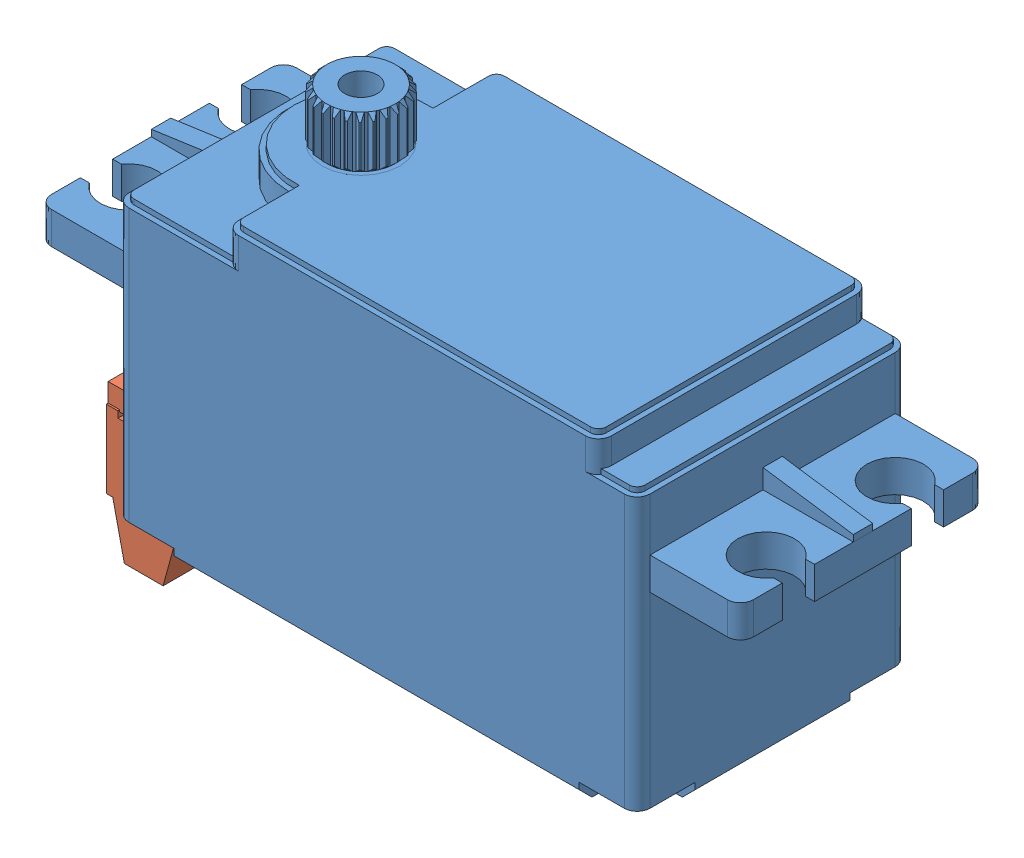
SolidWorks assembly OWServoAssem, configuration Default. Lengths in mm.
Overall size (54.6 37.3 21).
2 component instances, 2 part files, 3 mates.
Components (placement in the parent):
- HS-8775MG-1: HS-8775MG [Default] at (-15.3347 -5.6022 1.5156) size (54.4 29.4 21)
- OWServo-1: OWServo [Default] at (-56.0347 -2.0522 -166.4844) x (0 0 1) z (0 -1 0) size (17 46 16.9)
Mates (geometry in assembly coordinates):
- Width1: width aligned: plane of HS-8775MG-1 through (-14.8347 -5.6022 2.0156) normal (0 0 1); plane of OWServo-1 through (23.5653 -5.6022 -18.9844) normal (0 0 -1); plane of HS-8775MG-1 through (10.4653 -2.0522 -0.4844) normal (0 0 1); plane of OWServo-1 through (-7.4347 -2.0522 -16.4844) normal (0 0 -1)
- Width2: width anti-aligned: plane of HS-8775MG-1 through (-21.8347 -2.1022 -10.4844) normal (0 -1 0); plane of OWServo-1 through (-21.8347 -3.6022 -6.4844) normal (0 1 0); plane of HS-8775MG-1 through (-0.7021 -2.0522 -8.5058) normal (0 1 0); plane of OWServo-1 through (-0.7021 -3.6522 -8.5058) normal (0 -1 0)
- Distance8: distance = 1.6 mm: point of OWServo-1; plane of HS-8775MG-1 through (24.5653 -5.6022 1.0156) normal (1 0 0)
